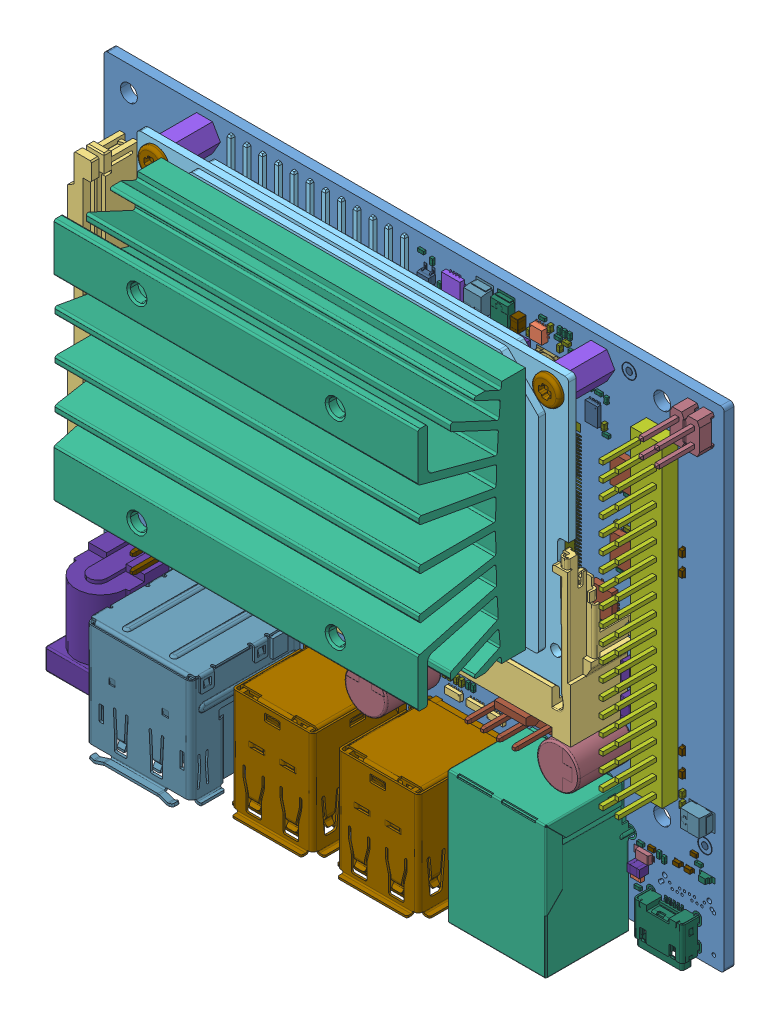
SolidWorks assembly Jetson_Nano_Dev_Kit_3D_b01, configuration Default. Lengths in mm.
Overall size (100 81.03 30.51).
406 component instances, 82 part files, 0 mates.
Components (placement in the parent):
- Jetson_Nano_Dev_Kit_3D_b01(2)^Jetson_Nano_Dev_Kit_3D_b01-1: Jetson_Nano_Dev_Kit_3D_b01(2)^Jetson_Nano_Dev_Kit_3D_b01 [Default] at origin size (100 81.03 30.51) (virtual)
  - 642-13450_PORG_SYS_BOM^Jetson_Nano_Dev_Kit_3D_b01(2)_Jetson_Nano_Dev_Kit_3D_b01-1: 642-13450_PORG_SYS_BOM^Jetson_Nano_Dev_Kit_3D_b01(2)_Jetson_Nano_Dev_Kit_3D_b01 [Default] at origin size (100 81.03 23.18) (virtual)
    - 699-13449_PORG_DEV_KIT_PCB_ASSY^642-13450_PORG_SYS_BOM_Jetson_Nano_Dev_Kit_3D_b01(2)_Jetson_Nano_Dev_Kit_3D_b01-1: 699-13449_PORG_DEV_KIT_PCB_ASSY^642-13450_PORG_SYS_BOM_Jetson_Nano_Dev_Kit_3D_b01(2)_Jetson_Nano_Dev_Kit_3D_b01 [Default] at origin size (100 81.03 23.18) (virtual)
      - 600-13449_PORG_DEV_KIT_PCB_ASSY^699-13449_PORG_DEV_KIT_PCB_ASSY_642-13450_PORG_SYS_BOM_Jetson_Nano_Dev_Kit_3D_b01(2)_Jetson_Nano_Dev_Kit_3D_b01-1: 600-13449_PORG_DEV_KIT_PCB_ASSY^699-13449_PORG_DEV_KIT_PCB_ASSY_642-13450_PORG_SYS_BOM_Jetson_Nano_Dev_Kit_3D_b01(2)_Jetson_Nano_Dev_Kit_3D_b01 [Default] at origin size (100 81.03 23.18) (virtual)
        - 142-13449-1000-B01-SKU0000^600-13449_PORG_DEV_KIT_PCB_ASSY_699-13449_PORG_DEV_KIT_PCB_ASSY_642-13450_PORG_SYS_BOM_Jetson_Nano_Dev_Kit_3D_b01(2)_Jetson_Nano_Dev_Kit_3D_b01-1: 142-13449-1000-B01-SKU0000^600-13449_PORG_DEV_KIT_PCB_ASSY_699-13449_PORG_DEV_KIT_PCB_ASSY_642-13450_PORG_SYS_BOM_Jetson_Nano_Dev_Kit_3D_b01(2)_Jetson_Nano_Dev_Kit_3D_b01 [Default] at origin size (100 81.03 23.18) (virtual)
          - 142-13449-1000-B01-SKU0000-0^142-13449-1000-B01-SKU0000_600-13449_PORG_DEV_KIT_PCB_ASSY_699-13449_PORG_DEV_KIT_PCB_ASSY_642-13450_PORG_SYS_BOM_Jetson_Nano_Dev_Kit_3D_b01(2)_Jetson_Nano_Dev_Kit~-1: 142-13449-1000-B01-SKU0000-0^142-13449-1000-B01-SKU0000_600-13449_PORG_DEV_KIT_PCB_ASSY_699-13449_PORG_DEV_KIT_PCB_ASSY_642-13450_PORG_SYS_BOM_Jetson_Nano_Dev_Kit_3D_b01(2)_Jetson_Nano_Dev_Kit~ [Default] at origin size (100 79 1.57) (virtual)
          - 316-0613-000_2^142-13449-1000-B01-SKU0000_600-13449_PORG_DEV_KIT_PCB_ASSY_699-13449_PORG_DEV_KIT_PCB_ASSY_642-13450_PORG_SYS_BOM_Jetson_Nano_Dev_Kit_3D_b01(2)_Jetson_Nano_Dev_Kit_3D_b01-1: 316-0613-000_2^142-13449-1000-B01-SKU0000_600-13449_PORG_DEV_KIT_PCB_ASSY_699-13449_PORG_DEV_KIT_PCB_ASSY_642-13450_PORG_SYS_BOM_Jetson_Nano_Dev_Kit_3D_b01(2)_Jetson_Nano_Dev_Kit_3D_b01 [Default] at (66.65 58.1 1.57) x (0 -1 0) z (0 0 1) size (2.5 2.5 1) (virtual)
          - 080-1656-000_3^142-13449-1000-B01-SKU0000_600-13449_PORG_DEV_KIT_PCB_ASSY_699-13449_PORG_DEV_KIT_PCB_ASSY_642-13450_PORG_SYS_BOM_Jetson_Nano_Dev_Kit_3D_b01(2)_Jetson_Nano_Dev_Kit_3D_b01-1: 080-1656-000_3^142-13449-1000-B01-SKU0000_600-13449_PORG_DEV_KIT_PCB_ASSY_699-13449_PORG_DEV_KIT_PCB_ASSY_642-13450_PORG_SYS_BOM_Jetson_Nano_Dev_Kit_3D_b01(2)_Jetson_Nano_Dev_Kit_3D_b01 [Default] at (44 16.6 1.57) x (-1 0 0) z (0 0 1) size (77.5 25.85 9.66) (virtual)
          - 300-1128-000_1^142-13449-1000-B01-SKU0000_600-13449_PORG_DEV_KIT_PCB_ASSY_699-13449_PORG_DEV_KIT_PCB_ASSY_642-13450_PORG_SYS_BOM_Jetson_Nano_Dev_Kit_3D_b01(2)_Jetson_Nano_Dev_Kit_3D_b01-1: 300-1128-000_1^142-13449-1000-B01-SKU0000_600-13449_PORG_DEV_KIT_PCB_ASSY_699-13449_PORG_DEV_KIT_PCB_ASSY_642-13450_PORG_SYS_BOM_Jetson_Nano_Dev_Kit_3D_b01(2)_Jetson_Nano_Dev_Kit_3D_b01 [Default] at (22.85 5.75 1.57) x (-1 0 0) z (0 0 1) size (2.1 2.8 1.1) (virtual)
          - 300-1128-000_1^142-13449-1000-B01-SKU0000_600-13449_PORG_DEV_KIT_PCB_ASSY_699-13449_PORG_DEV_KIT_PCB_ASSY_642-13450_PORG_SYS_BOM_Jetson_Nano_Dev_Kit_3D_b01(2)_Jetson_Nano_Dev_Kit_3D_b01-2: 300-1128-000_1^142-13449-1000-B01-SKU0000_600-13449_PORG_DEV_KIT_PCB_ASSY_699-13449_PORG_DEV_KIT_PCB_ASSY_642-13450_PORG_SYS_BOM_Jetson_Nano_Dev_Kit_3D_b01(2)_Jetson_Nano_Dev_Kit_3D_b01 [Default] at (34.9 9.55 1.57) x (0 -1 0) z (0 0 1) size (2.1 2.8 1.1) (virtual)
          - 074-0239-000_1^142-13449-1000-B01-SKU0000_600-13449_PORG_DEV_KIT_PCB_ASSY_699-13449_PORG_DEV_KIT_PCB_ASSY_642-13450_PORG_SYS_BOM_Jetson_Nano_Dev_Kit_3D_b01(2)_Jetson_Nano_Dev_Kit_3D_b01-1: 074-0239-000_1^142-13449-1000-B01-SKU0000_600-13449_PORG_DEV_KIT_PCB_ASSY_699-13449_PORG_DEV_KIT_PCB_ASSY_642-13450_PORG_SYS_BOM_Jetson_Nano_Dev_Kit_3D_b01(2)_Jetson_Nano_Dev_Kit_3D_b01 [Default] at (31.71 54.5 1.57) x (-1 0 0) z (0 0 1) size (30.48 10.8 5.5) (virtual)
          - 115-0655-000_3^142-13449-1000-B01-SKU0000_600-13449_PORG_DEV_KIT_PCB_ASSY_699-13449_PORG_DEV_KIT_PCB_ASSY_642-13450_PORG_SYS_BOM_Jetson_Nano_Dev_Kit_3D_b01(2)_Jetson_Nano_Dev_Kit_3D_b01-1: 115-0655-000_3^142-13449-1000-B01-SKU0000_600-13449_PORG_DEV_KIT_PCB_ASSY_699-13449_PORG_DEV_KIT_PCB_ASSY_642-13450_PORG_SYS_BOM_Jetson_Nano_Dev_Kit_3D_b01(2)_Jetson_Nano_Dev_Kit_3D_b01 [Default] at (7.45 49.75 1.57) x (0 -1 0) z (0 0 1) size (2.3 1.9 0.55) (virtual)
          - 315-1117-000_1^142-13449-1000-B01-SKU0000_600-13449_PORG_DEV_KIT_PCB_ASSY_699-13449_PORG_DEV_KIT_PCB_ASSY_642-13450_PORG_SYS_BOM_Jetson_Nano_Dev_Kit_3D_b01(2)_Jetson_Nano_Dev_Kit_3D_b01-1: 315-1117-000_1^142-13449-1000-B01-SKU0000_600-13449_PORG_DEV_KIT_PCB_ASSY_699-13449_PORG_DEV_KIT_PCB_ASSY_642-13450_PORG_SYS_BOM_Jetson_Nano_Dev_Kit_3D_b01(2)_Jetson_Nano_Dev_Kit_3D_b01 [Default] at (56.3 6.6 1.57) x (0 1 0) z (0 0 1) size (2 2.5 0.8) (virtual)
          - 315-1109-000_1^142-13449-1000-B01-SKU0000_600-13449_PORG_DEV_KIT_PCB_ASSY_699-13449_PORG_DEV_KIT_PCB_ASSY_642-13450_PORG_SYS_BOM_Jetson_Nano_Dev_Kit_3D_b01(2)_Jetson_Nano_Dev_Kit_3D_b01-1: 315-1109-000_1^142-13449-1000-B01-SKU0000_600-13449_PORG_DEV_KIT_PCB_ASSY_699-13449_PORG_DEV_KIT_PCB_ASSY_642-13450_PORG_SYS_BOM_Jetson_Nano_Dev_Kit_3D_b01(2)_Jetson_Nano_Dev_Kit_3D_b01 [Default] at (52.75 57.1 1.57) x (0 1 0) z (0 0 1) size (4.5 3.5 0.8) (virtual)
          - 315-1109-000_1^142-13449-1000-B01-SKU0000_600-13449_PORG_DEV_KIT_PCB_ASSY_699-13449_PORG_DEV_KIT_PCB_ASSY_642-13450_PORG_SYS_BOM_Jetson_Nano_Dev_Kit_3D_b01(2)_Jetson_Nano_Dev_Kit_3D_b01-2: 315-1109-000_1^142-13449-1000-B01-SKU0000_600-13449_PORG_DEV_KIT_PCB_ASSY_699-13449_PORG_DEV_KIT_PCB_ASSY_642-13450_PORG_SYS_BOM_Jetson_Nano_Dev_Kit_3D_b01(2)_Jetson_Nano_Dev_Kit_3D_b01 [Default] at (55.1 51.05 1.57) x (0 1 0) z (0 0 1) size (4.5 3.5 0.8) (virtual)
          - 115-2628-000_3^142-13449-1000-B01-SKU0000_600-13449_PORG_DEV_KIT_PCB_ASSY_699-13449_PORG_DEV_KIT_PCB_ASSY_642-13450_PORG_SYS_BOM_Jetson_Nano_Dev_Kit_3D_b01(2)_Jetson_Nano_Dev_Kit_3D_b01-1: 115-2628-000_3^142-13449-1000-B01-SKU0000_600-13449_PORG_DEV_KIT_PCB_ASSY_699-13449_PORG_DEV_KIT_PCB_ASSY_642-13450_PORG_SYS_BOM_Jetson_Nano_Dev_Kit_3D_b01(2)_Jetson_Nano_Dev_Kit_3D_b01 [Default] at (23.7 35.2 1.57) size (9.5 9.5 0.9) (virtual)
          - 174-0159-000_2^142-13449-1000-B01-SKU0000_600-13449_PORG_DEV_KIT_PCB_ASSY_699-13449_PORG_DEV_KIT_PCB_ASSY_642-13450_PORG_SYS_BOM_Jetson_Nano_Dev_Kit_3D_b01(2)_Jetson_Nano_Dev_Kit_3D_b01-1: 174-0159-000_2^142-13449-1000-B01-SKU0000_600-13449_PORG_DEV_KIT_PCB_ASSY_699-13449_PORG_DEV_KIT_PCB_ASSY_642-13450_PORG_SYS_BOM_Jetson_Nano_Dev_Kit_3D_b01(2)_Jetson_Nano_Dev_Kit_3D_b01 [Default] at (75.24 51.1 1.57) x (-1 0 0) z (0 0 1) size (2 3.52 0.6) (virtual)
          - 064-0400-000_1^142-13449-1000-B01-SKU0000_600-13449_PORG_DEV_KIT_PCB_ASSY_699-13449_PORG_DEV_KIT_PCB_ASSY_642-13450_PORG_SYS_BOM_Jetson_Nano_Dev_Kit_3D_b01(2)_Jetson_Nano_Dev_Kit_3D_b01-1: 064-0400-000_1^142-13449-1000-B01-SKU0000_600-13449_PORG_DEV_KIT_PCB_ASSY_699-13449_PORG_DEV_KIT_PCB_ASSY_642-13450_PORG_SYS_BOM_Jetson_Nano_Dev_Kit_3D_b01(2)_Jetson_Nano_Dev_Kit_3D_b01 [Default] at (68.2 7.77 1.57) size (10.16 5.8 13.5) (virtual)
          - 130-0938-000_1^142-13449-1000-B01-SKU0000_600-13449_PORG_DEV_KIT_PCB_ASSY_699-13449_PORG_DEV_KIT_PCB_ASSY_642-13450_PORG_SYS_BOM_Jetson_Nano_Dev_Kit_3D_b01(2)_Jetson_Nano_Dev_Kit_3D_b01-1: 130-0938-000_1^142-13449-1000-B01-SKU0000_600-13449_PORG_DEV_KIT_PCB_ASSY_699-13449_PORG_DEV_KIT_PCB_ASSY_642-13450_PORG_SYS_BOM_Jetson_Nano_Dev_Kit_3D_b01(2)_Jetson_Nano_Dev_Kit_3D_b01 [Default] at (68.05 53.85 1.57) x (-1 0 0) z (0 0 1) size (4.4 4 2) (virtual)
          - 032-1441-000_1^142-13449-1000-B01-SKU0000_600-13449_PORG_DEV_KIT_PCB_ASSY_699-13449_PORG_DEV_KIT_PCB_ASSY_642-13450_PORG_SYS_BOM_Jetson_Nano_Dev_Kit_3D_b01(2)_Jetson_Nano_Dev_Kit_3D_b01-1: 032-1441-000_1^142-13449-1000-B01-SKU0000_600-13449_PORG_DEV_KIT_PCB_ASSY_699-13449_PORG_DEV_KIT_PCB_ASSY_642-13450_PORG_SYS_BOM_Jetson_Nano_Dev_Kit_3D_b01(2)_Jetson_Nano_Dev_Kit_3D_b01 [Default] at (78.12 7.4 1.57) size (6.8 6.8 12.5) (virtual)
          - 032-1441-000_1^142-13449-1000-B01-SKU0000_600-13449_PORG_DEV_KIT_PCB_ASSY_699-13449_PORG_DEV_KIT_PCB_ASSY_642-13450_PORG_SYS_BOM_Jetson_Nano_Dev_Kit_3D_b01(2)_Jetson_Nano_Dev_Kit_3D_b01-2: 032-1441-000_1^142-13449-1000-B01-SKU0000_600-13449_PORG_DEV_KIT_PCB_ASSY_699-13449_PORG_DEV_KIT_PCB_ASSY_642-13450_PORG_SYS_BOM_Jetson_Nano_Dev_Kit_3D_b01(2)_Jetson_Nano_Dev_Kit_3D_b01 [Default] at (47.1 2.4 1.57) x (0 1 0) z (0 0 1) size (6.8 6.8 12.5) (virtual)
          - 090-0377-000_1^142-13449-1000-B01-SKU0000_600-13449_PORG_DEV_KIT_PCB_ASSY_699-13449_PORG_DEV_KIT_PCB_ASSY_642-13450_PORG_SYS_BOM_Jetson_Nano_Dev_Kit_3D_b01(2)_Jetson_Nano_Dev_Kit_3D_b01-1: 090-0377-000_1^142-13449-1000-B01-SKU0000_600-13449_PORG_DEV_KIT_PCB_ASSY_699-13449_PORG_DEV_KIT_PCB_ASSY_642-13450_PORG_SYS_BOM_Jetson_Nano_Dev_Kit_3D_b01(2)_Jetson_Nano_Dev_Kit_3D_b01 [Default] at (5.55 2.75 1.57) size (3 1.25 0.75) (virtual)
          - 0402_H040^142-13449-1000-B01-SKU0000_600-13449_PORG_DEV_KIT_PCB_ASSY_699-13449_PORG_DEV_KIT_PCB_ASSY_642-13450_PORG_SYS_BOM_Jetson_Nano_Dev_Kit_3D_b01(2)_Jetson_Nano_Dev_Kit_3D_b01-1: 0402_H040^142-13449-1000-B01-SKU0000_600-13449_PORG_DEV_KIT_PCB_ASSY_699-13449_PORG_DEV_KIT_PCB_ASSY_642-13450_PORG_SYS_BOM_Jetson_Nano_Dev_Kit_3D_b01(2)_Jetson_Nano_Dev_Kit_3D_b01 [Default] at (61.45 4.8 1.57) x (0 -1 0) z (0 0 1) size (1 0.5 0.4) (virtual)
          - 0402_H040^142-13449-1000-B01-SKU0000_600-13449_PORG_DEV_KIT_PCB_ASSY_699-13449_PORG_DEV_KIT_PCB_ASSY_642-13450_PORG_SYS_BOM_Jetson_Nano_Dev_Kit_3D_b01(2)_Jetson_Nano_Dev_Kit_3D_b01-2: 0402_H040^142-13449-1000-B01-SKU0000_600-13449_PORG_DEV_KIT_PCB_ASSY_699-13449_PORG_DEV_KIT_PCB_ASSY_642-13450_PORG_SYS_BOM_Jetson_Nano_Dev_Kit_3D_b01(2)_Jetson_Nano_Dev_Kit_3D_b01 [Default] at (71.9 4.1 1.57) x (-1 0 0) z (0 0 1) size (1 0.5 0.4) (virtual)
          - 0402_H040^142-13449-1000-B01-SKU0000_600-13449_PORG_DEV_KIT_PCB_ASSY_699-13449_PORG_DEV_KIT_PCB_ASSY_642-13450_PORG_SYS_BOM_Jetson_Nano_Dev_Kit_3D_b01(2)_Jetson_Nano_Dev_Kit_3D_b01-3: 0402_H040^142-13449-1000-B01-SKU0000_600-13449_PORG_DEV_KIT_PCB_ASSY_699-13449_PORG_DEV_KIT_PCB_ASSY_642-13450_PORG_SYS_BOM_Jetson_Nano_Dev_Kit_3D_b01(2)_Jetson_Nano_Dev_Kit_3D_b01 [Default] at (0.95 5.5 1.57) x (0 1 0) z (0 0 1) size (1 0.5 0.4) (virtual)
          - 0402_H040^142-13449-1000-B01-SKU0000_600-13449_PORG_DEV_KIT_PCB_ASSY_699-13449_PORG_DEV_KIT_PCB_ASSY_642-13450_PORG_SYS_BOM_Jetson_Nano_Dev_Kit_3D_b01(2)_Jetson_Nano_Dev_Kit_3D_b01-4: 0402_H040^142-13449-1000-B01-SKU0000_600-13449_PORG_DEV_KIT_PCB_ASSY_699-13449_PORG_DEV_KIT_PCB_ASSY_642-13450_PORG_SYS_BOM_Jetson_Nano_Dev_Kit_3D_b01(2)_Jetson_Nano_Dev_Kit_3D_b01 [Default] at (54.95 54.55 1.57) x (0 -1 0) z (0 0 1) size (1 0.5 0.4) (virtual)
          - 0402_H040^142-13449-1000-B01-SKU0000_600-13449_PORG_DEV_KIT_PCB_ASSY_699-13449_PORG_DEV_KIT_PCB_ASSY_642-13450_PORG_SYS_BOM_Jetson_Nano_Dev_Kit_3D_b01(2)_Jetson_Nano_Dev_Kit_3D_b01-5: 0402_H040^142-13449-1000-B01-SKU0000_600-13449_PORG_DEV_KIT_PCB_ASSY_699-13449_PORG_DEV_KIT_PCB_ASSY_642-13450_PORG_SYS_BOM_Jetson_Nano_Dev_Kit_3D_b01(2)_Jetson_Nano_Dev_Kit_3D_b01 [Default] at (55.75 54.55 1.57) x (0 1 0) z (0 0 1) size (1 0.5 0.4) (virtual)
          - 0402_H040^142-13449-1000-B01-SKU0000_600-13449_PORG_DEV_KIT_PCB_ASSY_699-13449_PORG_DEV_KIT_PCB_ASSY_642-13450_PORG_SYS_BOM_Jetson_Nano_Dev_Kit_3D_b01(2)_Jetson_Nano_Dev_Kit_3D_b01-6: 0402_H040^142-13449-1000-B01-SKU0000_600-13449_PORG_DEV_KIT_PCB_ASSY_699-13449_PORG_DEV_KIT_PCB_ASSY_642-13450_PORG_SYS_BOM_Jetson_Nano_Dev_Kit_3D_b01(2)_Jetson_Nano_Dev_Kit_3D_b01 [Default] at (35.75 7.8 1.57) x (-1 0 0) z (0 0 1) size (1 0.5 0.4) (virtual)
          - 0402_H040^142-13449-1000-B01-SKU0000_600-13449_PORG_DEV_KIT_PCB_ASSY_699-13449_PORG_DEV_KIT_PCB_ASSY_642-13450_PORG_SYS_BOM_Jetson_Nano_Dev_Kit_3D_b01(2)_Jetson_Nano_Dev_Kit_3D_b01-7: 0402_H040^142-13449-1000-B01-SKU0000_600-13449_PORG_DEV_KIT_PCB_ASSY_699-13449_PORG_DEV_KIT_PCB_ASSY_642-13450_PORG_SYS_BOM_Jetson_Nano_Dev_Kit_3D_b01(2)_Jetson_Nano_Dev_Kit_3D_b01 [Default] at (51.5 54.2 1.57) x (-1 0 0) z (0 0 1) size (1 0.5 0.4) (virtual)
          - 0402_H040^142-13449-1000-B01-SKU0000_600-13449_PORG_DEV_KIT_PCB_ASSY_699-13449_PORG_DEV_KIT_PCB_ASSY_642-13450_PORG_SYS_BOM_Jetson_Nano_Dev_Kit_3D_b01(2)_Jetson_Nano_Dev_Kit_3D_b01-8: 0402_H040^142-13449-1000-B01-SKU0000_600-13449_PORG_DEV_KIT_PCB_ASSY_699-13449_PORG_DEV_KIT_PCB_ASSY_642-13450_PORG_SYS_BOM_Jetson_Nano_Dev_Kit_3D_b01(2)_Jetson_Nano_Dev_Kit_3D_b01 [Default] at (47.5 59.85 1.57) size (1 0.5 0.4) (virtual)
          - 0402_H040^142-13449-1000-B01-SKU0000_600-13449_PORG_DEV_KIT_PCB_ASSY_699-13449_PORG_DEV_KIT_PCB_ASSY_642-13450_PORG_SYS_BOM_Jetson_Nano_Dev_Kit_3D_b01(2)_Jetson_Nano_Dev_Kit_3D_b01-9: 0402_H040^142-13449-1000-B01-SKU0000_600-13449_PORG_DEV_KIT_PCB_ASSY_699-13449_PORG_DEV_KIT_PCB_ASSY_642-13450_PORG_SYS_BOM_Jetson_Nano_Dev_Kit_3D_b01(2)_Jetson_Nano_Dev_Kit_3D_b01 [Default] at (50 54.8 1.57) x (-1 0 0) z (0 0 1) size (1 0.5 0.4) (virtual)
          - 0402_H040^142-13449-1000-B01-SKU0000_600-13449_PORG_DEV_KIT_PCB_ASSY_699-13449_PORG_DEV_KIT_PCB_ASSY_642-13450_PORG_SYS_BOM_Jetson_Nano_Dev_Kit_3D_b01(2)_Jetson_Nano_Dev_Kit_3D_b01-10: 0402_H040^142-13449-1000-B01-SKU0000_600-13449_PORG_DEV_KIT_PCB_ASSY_699-13449_PORG_DEV_KIT_PCB_ASSY_642-13450_PORG_SYS_BOM_Jetson_Nano_Dev_Kit_3D_b01(2)_Jetson_Nano_Dev_Kit_3D_b01 [Default] at (50.4 56.45 1.57) x (0 -1 0) z (0 0 1) size (1 0.5 0.4) (virtual)
          - 0402_H040^142-13449-1000-B01-SKU0000_600-13449_PORG_DEV_KIT_PCB_ASSY_699-13449_PORG_DEV_KIT_PCB_ASSY_642-13450_PORG_SYS_BOM_Jetson_Nano_Dev_Kit_3D_b01(2)_Jetson_Nano_Dev_Kit_3D_b01-11: 0402_H040^142-13449-1000-B01-SKU0000_600-13449_PORG_DEV_KIT_PCB_ASSY_699-13449_PORG_DEV_KIT_PCB_ASSY_642-13450_PORG_SYS_BOM_Jetson_Nano_Dev_Kit_3D_b01(2)_Jetson_Nano_Dev_Kit_3D_b01 [Default] at (49.2 59.25 1.57) x (0 -1 0) z (0 0 1) size (1 0.5 0.4) (virtual)
          - 0402_H040^142-13449-1000-B01-SKU0000_600-13449_PORG_DEV_KIT_PCB_ASSY_699-13449_PORG_DEV_KIT_PCB_ASSY_642-13450_PORG_SYS_BOM_Jetson_Nano_Dev_Kit_3D_b01(2)_Jetson_Nano_Dev_Kit_3D_b01-12: 0402_H040^142-13449-1000-B01-SKU0000_600-13449_PORG_DEV_KIT_PCB_ASSY_699-13449_PORG_DEV_KIT_PCB_ASSY_642-13450_PORG_SYS_BOM_Jetson_Nano_Dev_Kit_3D_b01(2)_Jetson_Nano_Dev_Kit_3D_b01 [Default] at (21.9 3.7 1.57) x (-1 0 0) z (0 0 1) size (1 0.5 0.4) (virtual)
          - 0402_H040^142-13449-1000-B01-SKU0000_600-13449_PORG_DEV_KIT_PCB_ASSY_699-13449_PORG_DEV_KIT_PCB_ASSY_642-13450_PORG_SYS_BOM_Jetson_Nano_Dev_Kit_3D_b01(2)_Jetson_Nano_Dev_Kit_3D_b01-13: 0402_H040^142-13449-1000-B01-SKU0000_600-13449_PORG_DEV_KIT_PCB_ASSY_699-13449_PORG_DEV_KIT_PCB_ASSY_642-13450_PORG_SYS_BOM_Jetson_Nano_Dev_Kit_3D_b01(2)_Jetson_Nano_Dev_Kit_3D_b01 [Default] at (23.5 3.7 1.57) size (1 0.5 0.4) (virtual)
          - 0402_H040^142-13449-1000-B01-SKU0000_600-13449_PORG_DEV_KIT_PCB_ASSY_699-13449_PORG_DEV_KIT_PCB_ASSY_642-13450_PORG_SYS_BOM_Jetson_Nano_Dev_Kit_3D_b01(2)_Jetson_Nano_Dev_Kit_3D_b01-14: 0402_H040^142-13449-1000-B01-SKU0000_600-13449_PORG_DEV_KIT_PCB_ASSY_699-13449_PORG_DEV_KIT_PCB_ASSY_642-13450_PORG_SYS_BOM_Jetson_Nano_Dev_Kit_3D_b01(2)_Jetson_Nano_Dev_Kit_3D_b01 [Default] at (34.6 7.4 1.57) x (0 1 0) z (0 0 1) size (1 0.5 0.4) (virtual)
          - 0402_H060^142-13449-1000-B01-SKU0000_600-13449_PORG_DEV_KIT_PCB_ASSY_699-13449_PORG_DEV_KIT_PCB_ASSY_642-13450_PORG_SYS_BOM_Jetson_Nano_Dev_Kit_3D_b01(2)_Jetson_Nano_Dev_Kit_3D_b01-1: 0402_H060^142-13449-1000-B01-SKU0000_600-13449_PORG_DEV_KIT_PCB_ASSY_699-13449_PORG_DEV_KIT_PCB_ASSY_642-13450_PORG_SYS_BOM_Jetson_Nano_Dev_Kit_3D_b01(2)_Jetson_Nano_Dev_Kit_3D_b01 [Default] at (53 54.2 1.57) size (1 0.5 0.6) (virtual)
          - 0402_H040^142-13449-1000-B01-SKU0000_600-13449_PORG_DEV_KIT_PCB_ASSY_699-13449_PORG_DEV_KIT_PCB_ASSY_642-13450_PORG_SYS_BOM_Jetson_Nano_Dev_Kit_3D_b01(2)_Jetson_Nano_Dev_Kit_3D_b01-15: 0402_H040^142-13449-1000-B01-SKU0000_600-13449_PORG_DEV_KIT_PCB_ASSY_699-13449_PORG_DEV_KIT_PCB_ASSY_642-13450_PORG_SYS_BOM_Jetson_Nano_Dev_Kit_3D_b01(2)_Jetson_Nano_Dev_Kit_3D_b01 [Default] at (44.8 45.25 1.57) size (1 0.5 0.4) (virtual)
          - 0402_H040^142-13449-1000-B01-SKU0000_600-13449_PORG_DEV_KIT_PCB_ASSY_699-13449_PORG_DEV_KIT_PCB_ASSY_642-13450_PORG_SYS_BOM_Jetson_Nano_Dev_Kit_3D_b01(2)_Jetson_Nano_Dev_Kit_3D_b01-16: 0402_H040^142-13449-1000-B01-SKU0000_600-13449_PORG_DEV_KIT_PCB_ASSY_699-13449_PORG_DEV_KIT_PCB_ASSY_642-13450_PORG_SYS_BOM_Jetson_Nano_Dev_Kit_3D_b01(2)_Jetson_Nano_Dev_Kit_3D_b01 [Default] at (44.8 44.45 1.57) size (1 0.5 0.4) (virtual)
          - 0402_H040^142-13449-1000-B01-SKU0000_600-13449_PORG_DEV_KIT_PCB_ASSY_699-13449_PORG_DEV_KIT_PCB_ASSY_642-13450_PORG_SYS_BOM_Jetson_Nano_Dev_Kit_3D_b01(2)_Jetson_Nano_Dev_Kit_3D_b01-17: 0402_H040^142-13449-1000-B01-SKU0000_600-13449_PORG_DEV_KIT_PCB_ASSY_699-13449_PORG_DEV_KIT_PCB_ASSY_642-13450_PORG_SYS_BOM_Jetson_Nano_Dev_Kit_3D_b01(2)_Jetson_Nano_Dev_Kit_3D_b01 [Default] at (54.15 25.3 1.57) size (1 0.5 0.4) (virtual)
          - 0402_H040^142-13449-1000-B01-SKU0000_600-13449_PORG_DEV_KIT_PCB_ASSY_699-13449_PORG_DEV_KIT_PCB_ASSY_642-13450_PORG_SYS_BOM_Jetson_Nano_Dev_Kit_3D_b01(2)_Jetson_Nano_Dev_Kit_3D_b01-18: 0402_H040^142-13449-1000-B01-SKU0000_600-13449_PORG_DEV_KIT_PCB_ASSY_699-13449_PORG_DEV_KIT_PCB_ASSY_642-13450_PORG_SYS_BOM_Jetson_Nano_Dev_Kit_3D_b01(2)_Jetson_Nano_Dev_Kit_3D_b01 [Default] at (9.35 48.95 1.57) x (0 1 0) z (0 0 1) size (1 0.5 0.4) (virtual)
          - 0402_H040^142-13449-1000-B01-SKU0000_600-13449_PORG_DEV_KIT_PCB_ASSY_699-13449_PORG_DEV_KIT_PCB_ASSY_642-13450_PORG_SYS_BOM_Jetson_Nano_Dev_Kit_3D_b01(2)_Jetson_Nano_Dev_Kit_3D_b01-19: 0402_H040^142-13449-1000-B01-SKU0000_600-13449_PORG_DEV_KIT_PCB_ASSY_699-13449_PORG_DEV_KIT_PCB_ASSY_642-13450_PORG_SYS_BOM_Jetson_Nano_Dev_Kit_3D_b01(2)_Jetson_Nano_Dev_Kit_3D_b01 [Default] at (9.35 50.45 1.57) x (0 -1 0) z (0 0 1) size (1 0.5 0.4) (virtual)
          - 0402_H040^142-13449-1000-B01-SKU0000_600-13449_PORG_DEV_KIT_PCB_ASSY_699-13449_PORG_DEV_KIT_PCB_ASSY_642-13450_PORG_SYS_BOM_Jetson_Nano_Dev_Kit_3D_b01(2)_Jetson_Nano_Dev_Kit_3D_b01-20: 0402_H040^142-13449-1000-B01-SKU0000_600-13449_PORG_DEV_KIT_PCB_ASSY_699-13449_PORG_DEV_KIT_PCB_ASSY_642-13450_PORG_SYS_BOM_Jetson_Nano_Dev_Kit_3D_b01(2)_Jetson_Nano_Dev_Kit_3D_b01 [Default] at (5.55 48.85 1.57) x (0 1 0) z (0 0 1) size (1 0.5 0.4) (virtual)
          - 0402_H040^142-13449-1000-B01-SKU0000_600-13449_PORG_DEV_KIT_PCB_ASSY_699-13449_PORG_DEV_KIT_PCB_ASSY_642-13450_PORG_SYS_BOM_Jetson_Nano_Dev_Kit_3D_b01(2)_Jetson_Nano_Dev_Kit_3D_b01-21: 0402_H040^142-13449-1000-B01-SKU0000_600-13449_PORG_DEV_KIT_PCB_ASSY_699-13449_PORG_DEV_KIT_PCB_ASSY_642-13450_PORG_SYS_BOM_Jetson_Nano_Dev_Kit_3D_b01(2)_Jetson_Nano_Dev_Kit_3D_b01 [Default] at (8.5 51.9 1.57) size (1 0.5 0.4) (virtual)
          - 0402_H040^142-13449-1000-B01-SKU0000_600-13449_PORG_DEV_KIT_PCB_ASSY_699-13449_PORG_DEV_KIT_PCB_ASSY_642-13450_PORG_SYS_BOM_Jetson_Nano_Dev_Kit_3D_b01(2)_Jetson_Nano_Dev_Kit_3D_b01-22: 0402_H040^142-13449-1000-B01-SKU0000_600-13449_PORG_DEV_KIT_PCB_ASSY_699-13449_PORG_DEV_KIT_PCB_ASSY_642-13450_PORG_SYS_BOM_Jetson_Nano_Dev_Kit_3D_b01(2)_Jetson_Nano_Dev_Kit_3D_b01 [Default] at (5.55 50.45 1.57) x (0 -1 0) z (0 0 1) size (1 0.5 0.4) (virtual)
          - 0402_H040^142-13449-1000-B01-SKU0000_600-13449_PORG_DEV_KIT_PCB_ASSY_699-13449_PORG_DEV_KIT_PCB_ASSY_642-13450_PORG_SYS_BOM_Jetson_Nano_Dev_Kit_3D_b01(2)_Jetson_Nano_Dev_Kit_3D_b01-23: 0402_H040^142-13449-1000-B01-SKU0000_600-13449_PORG_DEV_KIT_PCB_ASSY_699-13449_PORG_DEV_KIT_PCB_ASSY_642-13450_PORG_SYS_BOM_Jetson_Nano_Dev_Kit_3D_b01(2)_Jetson_Nano_Dev_Kit_3D_b01 [Default] at (6.45 51.9 1.57) x (-1 0 0) z (0 0 1) size (1 0.5 0.4) (virtual)
          - 0402_H040^142-13449-1000-B01-SKU0000_600-13449_PORG_DEV_KIT_PCB_ASSY_699-13449_PORG_DEV_KIT_PCB_ASSY_642-13450_PORG_SYS_BOM_Jetson_Nano_Dev_Kit_3D_b01(2)_Jetson_Nano_Dev_Kit_3D_b01-24: 0402_H040^142-13449-1000-B01-SKU0000_600-13449_PORG_DEV_KIT_PCB_ASSY_699-13449_PORG_DEV_KIT_PCB_ASSY_642-13450_PORG_SYS_BOM_Jetson_Nano_Dev_Kit_3D_b01(2)_Jetson_Nano_Dev_Kit_3D_b01 [Default] at (58.55 5.95 1.57) x (0 1 0) z (0 0 1) size (1 0.5 0.4) (virtual)
          - 0402_H060^142-13449-1000-B01-SKU0000_600-13449_PORG_DEV_KIT_PCB_ASSY_699-13449_PORG_DEV_KIT_PCB_ASSY_642-13450_PORG_SYS_BOM_Jetson_Nano_Dev_Kit_3D_b01(2)_Jetson_Nano_Dev_Kit_3D_b01-2: 0402_H060^142-13449-1000-B01-SKU0000_600-13449_PORG_DEV_KIT_PCB_ASSY_699-13449_PORG_DEV_KIT_PCB_ASSY_642-13450_PORG_SYS_BOM_Jetson_Nano_Dev_Kit_3D_b01(2)_Jetson_Nano_Dev_Kit_3D_b01 [Default] at (56.9 8.3 1.57) x (-1 0 0) z (0 0 1) size (1 0.5 0.6) (virtual)
          - 0402_H060^142-13449-1000-B01-SKU0000_600-13449_PORG_DEV_KIT_PCB_ASSY_699-13449_PORG_DEV_KIT_PCB_ASSY_642-13450_PORG_SYS_BOM_Jetson_Nano_Dev_Kit_3D_b01(2)_Jetson_Nano_Dev_Kit_3D_b01-3: 0402_H060^142-13449-1000-B01-SKU0000_600-13449_PORG_DEV_KIT_PCB_ASSY_699-13449_PORG_DEV_KIT_PCB_ASSY_642-13450_PORG_SYS_BOM_Jetson_Nano_Dev_Kit_3D_b01(2)_Jetson_Nano_Dev_Kit_3D_b01 [Default] at (57 4.9 1.57) size (1 0.5 0.6) (virtual)
          - 0402_H040^142-13449-1000-B01-SKU0000_600-13449_PORG_DEV_KIT_PCB_ASSY_699-13449_PORG_DEV_KIT_PCB_ASSY_642-13450_PORG_SYS_BOM_Jetson_Nano_Dev_Kit_3D_b01(2)_Jetson_Nano_Dev_Kit_3D_b01-25: 0402_H040^142-13449-1000-B01-SKU0000_600-13449_PORG_DEV_KIT_PCB_ASSY_699-13449_PORG_DEV_KIT_PCB_ASSY_642-13450_PORG_SYS_BOM_Jetson_Nano_Dev_Kit_3D_b01(2)_Jetson_Nano_Dev_Kit_3D_b01 [Default] at (48.15 54.8 1.57) size (1 0.5 0.4) (virtual)
          - 0402_H040^142-13449-1000-B01-SKU0000_600-13449_PORG_DEV_KIT_PCB_ASSY_699-13449_PORG_DEV_KIT_PCB_ASSY_642-13450_PORG_SYS_BOM_Jetson_Nano_Dev_Kit_3D_b01(2)_Jetson_Nano_Dev_Kit_3D_b01-26: 0402_H040^142-13449-1000-B01-SKU0000_600-13449_PORG_DEV_KIT_PCB_ASSY_699-13449_PORG_DEV_KIT_PCB_ASSY_642-13450_PORG_SYS_BOM_Jetson_Nano_Dev_Kit_3D_b01(2)_Jetson_Nano_Dev_Kit_3D_b01 [Default] at (54.4 5.85 1.57) x (0 -1 0) z (0 0 1) size (1 0.5 0.4) (virtual)
          - 0402_H040^142-13449-1000-B01-SKU0000_600-13449_PORG_DEV_KIT_PCB_ASSY_699-13449_PORG_DEV_KIT_PCB_ASSY_642-13450_PORG_SYS_BOM_Jetson_Nano_Dev_Kit_3D_b01(2)_Jetson_Nano_Dev_Kit_3D_b01-27: 0402_H040^142-13449-1000-B01-SKU0000_600-13449_PORG_DEV_KIT_PCB_ASSY_699-13449_PORG_DEV_KIT_PCB_ASSY_642-13450_PORG_SYS_BOM_Jetson_Nano_Dev_Kit_3D_b01(2)_Jetson_Nano_Dev_Kit_3D_b01 [Default] at (45.3 49.5 1.57) x (-1 0 0) z (0 0 1) size (1 0.5 0.4) (virtual)
          - 0402_H040^142-13449-1000-B01-SKU0000_600-13449_PORG_DEV_KIT_PCB_ASSY_699-13449_PORG_DEV_KIT_PCB_ASSY_642-13450_PORG_SYS_BOM_Jetson_Nano_Dev_Kit_3D_b01(2)_Jetson_Nano_Dev_Kit_3D_b01-28: 0402_H040^142-13449-1000-B01-SKU0000_600-13449_PORG_DEV_KIT_PCB_ASSY_699-13449_PORG_DEV_KIT_PCB_ASSY_642-13450_PORG_SYS_BOM_Jetson_Nano_Dev_Kit_3D_b01(2)_Jetson_Nano_Dev_Kit_3D_b01 [Default] at (71.5 57.55 1.57) x (0 1 0) z (0 0 1) size (1 0.5 0.4) (virtual)
          - 0402_H060^142-13449-1000-B01-SKU0000_600-13449_PORG_DEV_KIT_PCB_ASSY_699-13449_PORG_DEV_KIT_PCB_ASSY_642-13450_PORG_SYS_BOM_Jetson_Nano_Dev_Kit_3D_b01(2)_Jetson_Nano_Dev_Kit_3D_b01-4: 0402_H060^142-13449-1000-B01-SKU0000_600-13449_PORG_DEV_KIT_PCB_ASSY_699-13449_PORG_DEV_KIT_PCB_ASSY_642-13450_PORG_SYS_BOM_Jetson_Nano_Dev_Kit_3D_b01(2)_Jetson_Nano_Dev_Kit_3D_b01 [Default] at (3.95 49.55 1.57) x (0 1 0) z (0 0 1) size (1 0.5 0.6) (virtual)
          - 0402_H040^142-13449-1000-B01-SKU0000_600-13449_PORG_DEV_KIT_PCB_ASSY_699-13449_PORG_DEV_KIT_PCB_ASSY_642-13450_PORG_SYS_BOM_Jetson_Nano_Dev_Kit_3D_b01(2)_Jetson_Nano_Dev_Kit_3D_b01-29: 0402_H040^142-13449-1000-B01-SKU0000_600-13449_PORG_DEV_KIT_PCB_ASSY_699-13449_PORG_DEV_KIT_PCB_ASSY_642-13450_PORG_SYS_BOM_Jetson_Nano_Dev_Kit_3D_b01(2)_Jetson_Nano_Dev_Kit_3D_b01 [Default] at (62.45 50.25 1.57) x (-1 0 0) z (0 0 1) size (1 0.5 0.4) (virtual)
          - 0402_H040^142-13449-1000-B01-SKU0000_600-13449_PORG_DEV_KIT_PCB_ASSY_699-13449_PORG_DEV_KIT_PCB_ASSY_642-13450_PORG_SYS_BOM_Jetson_Nano_Dev_Kit_3D_b01(2)_Jetson_Nano_Dev_Kit_3D_b01-30: 0402_H040^142-13449-1000-B01-SKU0000_600-13449_PORG_DEV_KIT_PCB_ASSY_699-13449_PORG_DEV_KIT_PCB_ASSY_642-13450_PORG_SYS_BOM_Jetson_Nano_Dev_Kit_3D_b01(2)_Jetson_Nano_Dev_Kit_3D_b01 [Default] at (70.55 59.85 1.57) x (0 1 0) z (0 0 1) size (1 0.5 0.4) (virtual)
          - 0402_H040^142-13449-1000-B01-SKU0000_600-13449_PORG_DEV_KIT_PCB_ASSY_699-13449_PORG_DEV_KIT_PCB_ASSY_642-13450_PORG_SYS_BOM_Jetson_Nano_Dev_Kit_3D_b01(2)_Jetson_Nano_Dev_Kit_3D_b01-31: 0402_H040^142-13449-1000-B01-SKU0000_600-13449_PORG_DEV_KIT_PCB_ASSY_699-13449_PORG_DEV_KIT_PCB_ASSY_642-13450_PORG_SYS_BOM_Jetson_Nano_Dev_Kit_3D_b01(2)_Jetson_Nano_Dev_Kit_3D_b01 [Default] at (69.5 58.7 1.57) size (1 0.5 0.4) (virtual)
          - 0402_H060^142-13449-1000-B01-SKU0000_600-13449_PORG_DEV_KIT_PCB_ASSY_699-13449_PORG_DEV_KIT_PCB_ASSY_642-13450_PORG_SYS_BOM_Jetson_Nano_Dev_Kit_3D_b01(2)_Jetson_Nano_Dev_Kit_3D_b01-5: 0402_H060^142-13449-1000-B01-SKU0000_600-13449_PORG_DEV_KIT_PCB_ASSY_699-13449_PORG_DEV_KIT_PCB_ASSY_642-13450_PORG_SYS_BOM_Jetson_Nano_Dev_Kit_3D_b01(2)_Jetson_Nano_Dev_Kit_3D_b01 [Default] at (64.95 57.3 1.57) x (0 -1 0) z (0 0 1) size (1 0.5 0.6) (virtual)
          - 0402_H060^142-13449-1000-B01-SKU0000_600-13449_PORG_DEV_KIT_PCB_ASSY_699-13449_PORG_DEV_KIT_PCB_ASSY_642-13450_PORG_SYS_BOM_Jetson_Nano_Dev_Kit_3D_b01(2)_Jetson_Nano_Dev_Kit_3D_b01-6: 0402_H060^142-13449-1000-B01-SKU0000_600-13449_PORG_DEV_KIT_PCB_ASSY_699-13449_PORG_DEV_KIT_PCB_ASSY_642-13450_PORG_SYS_BOM_Jetson_Nano_Dev_Kit_3D_b01(2)_Jetson_Nano_Dev_Kit_3D_b01 [Default] at (69.9 57.55 1.57) x (0 -1 0) z (0 0 1) size (1 0.5 0.6) (virtual)
          - 0402_H040^142-13449-1000-B01-SKU0000_600-13449_PORG_DEV_KIT_PCB_ASSY_699-13449_PORG_DEV_KIT_PCB_ASSY_642-13450_PORG_SYS_BOM_Jetson_Nano_Dev_Kit_3D_b01(2)_Jetson_Nano_Dev_Kit_3D_b01-32: 0402_H040^142-13449-1000-B01-SKU0000_600-13449_PORG_DEV_KIT_PCB_ASSY_699-13449_PORG_DEV_KIT_PCB_ASSY_642-13450_PORG_SYS_BOM_Jetson_Nano_Dev_Kit_3D_b01(2)_Jetson_Nano_Dev_Kit_3D_b01 [Default] at (71.35 59.85 1.57) x (0 1 0) z (0 0 1) size (1 0.5 0.4) (virtual)
          - 0402_H040^142-13449-1000-B01-SKU0000_600-13449_PORG_DEV_KIT_PCB_ASSY_699-13449_PORG_DEV_KIT_PCB_ASSY_642-13450_PORG_SYS_BOM_Jetson_Nano_Dev_Kit_3D_b01(2)_Jetson_Nano_Dev_Kit_3D_b01-33: 0402_H040^142-13449-1000-B01-SKU0000_600-13449_PORG_DEV_KIT_PCB_ASSY_699-13449_PORG_DEV_KIT_PCB_ASSY_642-13450_PORG_SYS_BOM_Jetson_Nano_Dev_Kit_3D_b01(2)_Jetson_Nano_Dev_Kit_3D_b01 [Default] at (67 60.2 1.57) size (1 0.5 0.4) (virtual)
          - 0402_H040^142-13449-1000-B01-SKU0000_600-13449_PORG_DEV_KIT_PCB_ASSY_699-13449_PORG_DEV_KIT_PCB_ASSY_642-13450_PORG_SYS_BOM_Jetson_Nano_Dev_Kit_3D_b01(2)_Jetson_Nano_Dev_Kit_3D_b01-34: 0402_H040^142-13449-1000-B01-SKU0000_600-13449_PORG_DEV_KIT_PCB_ASSY_699-13449_PORG_DEV_KIT_PCB_ASSY_642-13450_PORG_SYS_BOM_Jetson_Nano_Dev_Kit_3D_b01(2)_Jetson_Nano_Dev_Kit_3D_b01 [Default] at (69.75 59.85 1.57) x (0 -1 0) z (0 0 1) size (1 0.5 0.4) (virtual)
          - 0402_H060^142-13449-1000-B01-SKU0000_600-13449_PORG_DEV_KIT_PCB_ASSY_699-13449_PORG_DEV_KIT_PCB_ASSY_642-13450_PORG_SYS_BOM_Jetson_Nano_Dev_Kit_3D_b01(2)_Jetson_Nano_Dev_Kit_3D_b01-7: 0402_H060^142-13449-1000-B01-SKU0000_600-13449_PORG_DEV_KIT_PCB_ASSY_699-13449_PORG_DEV_KIT_PCB_ASSY_642-13450_PORG_SYS_BOM_Jetson_Nano_Dev_Kit_3D_b01(2)_Jetson_Nano_Dev_Kit_3D_b01 [Default] at (70.95 58.7 1.57) size (1 0.5 0.6) (virtual)
          - 0402_H040^142-13449-1000-B01-SKU0000_600-13449_PORG_DEV_KIT_PCB_ASSY_699-13449_PORG_DEV_KIT_PCB_ASSY_642-13450_PORG_SYS_BOM_Jetson_Nano_Dev_Kit_3D_b01(2)_Jetson_Nano_Dev_Kit_3D_b01-35: 0402_H040^142-13449-1000-B01-SKU0000_600-13449_PORG_DEV_KIT_PCB_ASSY_699-13449_PORG_DEV_KIT_PCB_ASSY_642-13450_PORG_SYS_BOM_Jetson_Nano_Dev_Kit_3D_b01(2)_Jetson_Nano_Dev_Kit_3D_b01 [Default] at (47 48.3 1.57) size (1 0.5 0.4) (virtual)
          - 0402_H040^142-13449-1000-B01-SKU0000_600-13449_PORG_DEV_KIT_PCB_ASSY_699-13449_PORG_DEV_KIT_PCB_ASSY_642-13450_PORG_SYS_BOM_Jetson_Nano_Dev_Kit_3D_b01(2)_Jetson_Nano_Dev_Kit_3D_b01-36: 0402_H040^142-13449-1000-B01-SKU0000_600-13449_PORG_DEV_KIT_PCB_ASSY_699-13449_PORG_DEV_KIT_PCB_ASSY_642-13450_PORG_SYS_BOM_Jetson_Nano_Dev_Kit_3D_b01(2)_Jetson_Nano_Dev_Kit_3D_b01 [Default] at (62.5 22.8 1.57) x (-1 0 0) z (0 0 1) size (1 0.5 0.4) (virtual)
          - 0402_H040^142-13449-1000-B01-SKU0000_600-13449_PORG_DEV_KIT_PCB_ASSY_699-13449_PORG_DEV_KIT_PCB_ASSY_642-13450_PORG_SYS_BOM_Jetson_Nano_Dev_Kit_3D_b01(2)_Jetson_Nano_Dev_Kit_3D_b01-37: 0402_H040^142-13449-1000-B01-SKU0000_600-13449_PORG_DEV_KIT_PCB_ASSY_699-13449_PORG_DEV_KIT_PCB_ASSY_642-13450_PORG_SYS_BOM_Jetson_Nano_Dev_Kit_3D_b01(2)_Jetson_Nano_Dev_Kit_3D_b01 [Default] at (2.95 9.65 1.57) x (0 1 0) z (0 0 1) size (1 0.5 0.4) (virtual)
          - 0402_H040^142-13449-1000-B01-SKU0000_600-13449_PORG_DEV_KIT_PCB_ASSY_699-13449_PORG_DEV_KIT_PCB_ASSY_642-13450_PORG_SYS_BOM_Jetson_Nano_Dev_Kit_3D_b01(2)_Jetson_Nano_Dev_Kit_3D_b01-38: 0402_H040^142-13449-1000-B01-SKU0000_600-13449_PORG_DEV_KIT_PCB_ASSY_699-13449_PORG_DEV_KIT_PCB_ASSY_642-13450_PORG_SYS_BOM_Jetson_Nano_Dev_Kit_3D_b01(2)_Jetson_Nano_Dev_Kit_3D_b01 [Default] at (7.8 9.55 1.57) x (0 -1 0) z (0 0 1) size (1 0.5 0.4) (virtual)
          - 0402_H040^142-13449-1000-B01-SKU0000_600-13449_PORG_DEV_KIT_PCB_ASSY_699-13449_PORG_DEV_KIT_PCB_ASSY_642-13450_PORG_SYS_BOM_Jetson_Nano_Dev_Kit_3D_b01(2)_Jetson_Nano_Dev_Kit_3D_b01-39: 0402_H040^142-13449-1000-B01-SKU0000_600-13449_PORG_DEV_KIT_PCB_ASSY_699-13449_PORG_DEV_KIT_PCB_ASSY_642-13450_PORG_SYS_BOM_Jetson_Nano_Dev_Kit_3D_b01(2)_Jetson_Nano_Dev_Kit_3D_b01 [Default] at (12.1 10.15 1.57) x (0 1 0) z (0 0 1) size (1 0.5 0.4) (virtual)
          - 0402_H040^142-13449-1000-B01-SKU0000_600-13449_PORG_DEV_KIT_PCB_ASSY_699-13449_PORG_DEV_KIT_PCB_ASSY_642-13450_PORG_SYS_BOM_Jetson_Nano_Dev_Kit_3D_b01(2)_Jetson_Nano_Dev_Kit_3D_b01-40: 0402_H040^142-13449-1000-B01-SKU0000_600-13449_PORG_DEV_KIT_PCB_ASSY_699-13449_PORG_DEV_KIT_PCB_ASSY_642-13450_PORG_SYS_BOM_Jetson_Nano_Dev_Kit_3D_b01(2)_Jetson_Nano_Dev_Kit_3D_b01 [Default] at (27.7 40.6 1.57) x (-1 0 0) z (0 0 1) size (1 0.5 0.4) (virtual)
          - 0402_H060^142-13449-1000-B01-SKU0000_600-13449_PORG_DEV_KIT_PCB_ASSY_699-13449_PORG_DEV_KIT_PCB_ASSY_642-13450_PORG_SYS_BOM_Jetson_Nano_Dev_Kit_3D_b01(2)_Jetson_Nano_Dev_Kit_3D_b01-8: 0402_H060^142-13449-1000-B01-SKU0000_600-13449_PORG_DEV_KIT_PCB_ASSY_699-13449_PORG_DEV_KIT_PCB_ASSY_642-13450_PORG_SYS_BOM_Jetson_Nano_Dev_Kit_3D_b01(2)_Jetson_Nano_Dev_Kit_3D_b01 [Default] at (14.35 52.85 1.57) size (1 0.5 0.6) (virtual)
          - 0402_H040^142-13449-1000-B01-SKU0000_600-13449_PORG_DEV_KIT_PCB_ASSY_699-13449_PORG_DEV_KIT_PCB_ASSY_642-13450_PORG_SYS_BOM_Jetson_Nano_Dev_Kit_3D_b01(2)_Jetson_Nano_Dev_Kit_3D_b01-41: 0402_H040^142-13449-1000-B01-SKU0000_600-13449_PORG_DEV_KIT_PCB_ASSY_699-13449_PORG_DEV_KIT_PCB_ASSY_642-13450_PORG_SYS_BOM_Jetson_Nano_Dev_Kit_3D_b01(2)_Jetson_Nano_Dev_Kit_3D_b01 [Default] at (57 47.8 1.57) x (0 -1 0) z (0 0 1) size (1 0.5 0.4) (virtual)
          - 0402_H040^142-13449-1000-B01-SKU0000_600-13449_PORG_DEV_KIT_PCB_ASSY_699-13449_PORG_DEV_KIT_PCB_ASSY_642-13450_PORG_SYS_BOM_Jetson_Nano_Dev_Kit_3D_b01(2)_Jetson_Nano_Dev_Kit_3D_b01-42: 0402_H040^142-13449-1000-B01-SKU0000_600-13449_PORG_DEV_KIT_PCB_ASSY_699-13449_PORG_DEV_KIT_PCB_ASSY_642-13450_PORG_SYS_BOM_Jetson_Nano_Dev_Kit_3D_b01(2)_Jetson_Nano_Dev_Kit_3D_b01 [Default] at (37.8 2.87 1.57) x (0 -1 0) z (0 0 1) size (1 0.5 0.4) (virtual)
          - 0402_H040^142-13449-1000-B01-SKU0000_600-13449_PORG_DEV_KIT_PCB_ASSY_699-13449_PORG_DEV_KIT_PCB_ASSY_642-13450_PORG_SYS_BOM_Jetson_Nano_Dev_Kit_3D_b01(2)_Jetson_Nano_Dev_Kit_3D_b01-43: 0402_H040^142-13449-1000-B01-SKU0000_600-13449_PORG_DEV_KIT_PCB_ASSY_699-13449_PORG_DEV_KIT_PCB_ASSY_642-13450_PORG_SYS_BOM_Jetson_Nano_Dev_Kit_3D_b01(2)_Jetson_Nano_Dev_Kit_3D_b01 [Default] at (38.6 2.87 1.57) x (0 -1 0) z (0 0 1) size (1 0.5 0.4) (virtual)
          - 0402_H060^142-13449-1000-B01-SKU0000_600-13449_PORG_DEV_KIT_PCB_ASSY_699-13449_PORG_DEV_KIT_PCB_ASSY_642-13450_PORG_SYS_BOM_Jetson_Nano_Dev_Kit_3D_b01(2)_Jetson_Nano_Dev_Kit_3D_b01-9: 0402_H060^142-13449-1000-B01-SKU0000_600-13449_PORG_DEV_KIT_PCB_ASSY_699-13449_PORG_DEV_KIT_PCB_ASSY_642-13450_PORG_SYS_BOM_Jetson_Nano_Dev_Kit_3D_b01(2)_Jetson_Nano_Dev_Kit_3D_b01 [Default] at (14.2 7.7 1.57) x (0 -1 0) z (0 0 1) size (1 0.5 0.6) (virtual)
          - 0402_H060^142-13449-1000-B01-SKU0000_600-13449_PORG_DEV_KIT_PCB_ASSY_699-13449_PORG_DEV_KIT_PCB_ASSY_642-13450_PORG_SYS_BOM_Jetson_Nano_Dev_Kit_3D_b01(2)_Jetson_Nano_Dev_Kit_3D_b01-10: 0402_H060^142-13449-1000-B01-SKU0000_600-13449_PORG_DEV_KIT_PCB_ASSY_699-13449_PORG_DEV_KIT_PCB_ASSY_642-13450_PORG_SYS_BOM_Jetson_Nano_Dev_Kit_3D_b01(2)_Jetson_Nano_Dev_Kit_3D_b01 [Default] at (17.1 37.15 1.57) x (-1 0 0) z (0 0 1) size (1 0.5 0.6) (virtual)
          - 0402_H060^142-13449-1000-B01-SKU0000_600-13449_PORG_DEV_KIT_PCB_ASSY_699-13449_PORG_DEV_KIT_PCB_ASSY_642-13450_PORG_SYS_BOM_Jetson_Nano_Dev_Kit_3D_b01(2)_Jetson_Nano_Dev_Kit_3D_b01-11: 0402_H060^142-13449-1000-B01-SKU0000_600-13449_PORG_DEV_KIT_PCB_ASSY_699-13449_PORG_DEV_KIT_PCB_ASSY_642-13450_PORG_SYS_BOM_Jetson_Nano_Dev_Kit_3D_b01(2)_Jetson_Nano_Dev_Kit_3D_b01 [Default] at (62.5 25.4 1.57) x (-1 0 0) z (0 0 1) size (1 0.5 0.6) (virtual)
          - 0402_H060^142-13449-1000-B01-SKU0000_600-13449_PORG_DEV_KIT_PCB_ASSY_699-13449_PORG_DEV_KIT_PCB_ASSY_642-13450_PORG_SYS_BOM_Jetson_Nano_Dev_Kit_3D_b01(2)_Jetson_Nano_Dev_Kit_3D_b01-12: 0402_H060^142-13449-1000-B01-SKU0000_600-13449_PORG_DEV_KIT_PCB_ASSY_699-13449_PORG_DEV_KIT_PCB_ASSY_642-13450_PORG_SYS_BOM_Jetson_Nano_Dev_Kit_3D_b01(2)_Jetson_Nano_Dev_Kit_3D_b01 [Default] at (63.65 49.05 1.57) x (-1 0 0) z (0 0 1) size (1 0.5 0.6) (virtual)
          - 0402_H040^142-13449-1000-B01-SKU0000_600-13449_PORG_DEV_KIT_PCB_ASSY_699-13449_PORG_DEV_KIT_PCB_ASSY_642-13450_PORG_SYS_BOM_Jetson_Nano_Dev_Kit_3D_b01(2)_Jetson_Nano_Dev_Kit_3D_b01-44: 0402_H040^142-13449-1000-B01-SKU0000_600-13449_PORG_DEV_KIT_PCB_ASSY_699-13449_PORG_DEV_KIT_PCB_ASSY_642-13450_PORG_SYS_BOM_Jetson_Nano_Dev_Kit_3D_b01(2)_Jetson_Nano_Dev_Kit_3D_b01 [Default] at (65.5 22.8 1.57) size (1 0.5 0.4) (virtual)
          - 0402_H060^142-13449-1000-B01-SKU0000_600-13449_PORG_DEV_KIT_PCB_ASSY_699-13449_PORG_DEV_KIT_PCB_ASSY_642-13450_PORG_SYS_BOM_Jetson_Nano_Dev_Kit_3D_b01(2)_Jetson_Nano_Dev_Kit_3D_b01-13: 0402_H060^142-13449-1000-B01-SKU0000_600-13449_PORG_DEV_KIT_PCB_ASSY_699-13449_PORG_DEV_KIT_PCB_ASSY_642-13450_PORG_SYS_BOM_Jetson_Nano_Dev_Kit_3D_b01(2)_Jetson_Nano_Dev_Kit_3D_b01 [Default] at (17.3 7.7 1.57) x (0 -1 0) z (0 0 1) size (1 0.5 0.6) (virtual)
